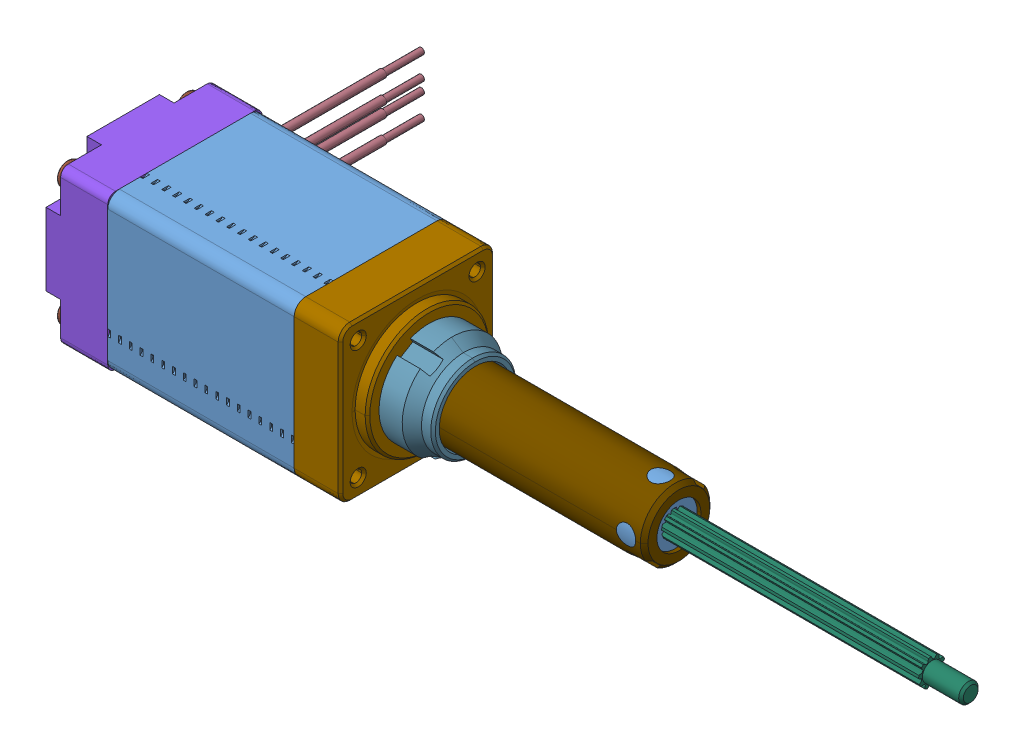
SolidWorks assembly 20NC38..31, configuration 默认. Lengths in mm.
Overall size (109.8 25.88 45.74).
31 component instances, 19 part files, 0 mates.
Components (placement in the parent):
- 20NC38..31.STEP-1: 20NC38..31.STEP [默认] at origin size (109.8 25.88 45.74)
  - 02-20-38.15________.STEP-1: 02-20-38.15________.STEP [默认] at origin size (39.65 25.88 45.74)
    - 02-20-38.STEP-1: 02-20-38.STEP [默认] at (20.075 0 0) x (0 0 1) z (-1 0 0) size (26.04 25.88 31.46)
      - 02-20-24.15_10-20-001-2.STEP-1: 02-20-24.15_10-20-001-2.STEP [默认] at origin size (20 20 24.15)
      - 13-20-8.5____.STEP-1: 13-20-8.5____.STEP [默认] at (0 0 16.075) x (0 1 0) z (0 0 -1) size (18.2 22.2 10.51)
      - 13-20-12.5______.STEP-1: 13-20-12.5______.STEP [默认] at (0 0 -14.575) x (0.707107 0.707107 0) z (0 0 1) size (18.3 18.3 15.8)
    - 03-20-008______38_______default.STEP-1: 03-20-008______38_______default.STEP [默认] at (3.8 0 0) x (1 0 0) z (0 0.78069 0.624918) size (32.3 16.26 16.27)
      - 06-20-008______38_________01-20-007-1.STEP-1: 06-20-008______38_________01-20-007-1.STEP [默认] at origin size (32.3 7 7)
      - 03-20-4.2-6YK_10-20-006-2.STEP-1: 03-20-4.2-6YK_10-20-006-2.STEP [默认] at (24.2 0 0) x (0 0.91534 0.402682) z (-1 0 0) size (12.06 12.08 4.2)
      - 10-20-001__________.STEP-1: 10-20-001__________.STEP [默认] at (16.9 0 0) x (0 0 1) z (-1 0 0) size (11.2 11.2 1.3)
      - 08-20-001______1_______07-20-001-1.STEP-1: 08-20-001______1_______07-20-001-1.STEP [默认] at (22.1 0 0) x (0 0 1) z (-1 0 0) size (11 11 1)
      - 08-20-001______1_______07-20-001-1.STEP-2: 08-20-001______1_______07-20-001-1.STEP [默认] at (11.4 0 0) x (0 0 1) z (-1 0 0) size (11 11 1)
      - 03-20-4.2-6YK_10-20-006-2.STEP-2: 03-20-4.2-6YK_10-20-006-2.STEP [默认] at (19 0 0) x (0 0.888249 0.459362) z (-1 0 0) size (12.06 12.08 4.2)
      - 03-20-4.2-6YK_10-20-006-2.STEP-3: 03-20-4.2-6YK_10-20-006-2.STEP [默认] at (13.5 0 0) x (0 0.91534 0.402682) z (-1 0 0) size (12.06 12.08 4.2)
      - 03-20-4.2-6YK_10-20-006-2.STEP-4: 03-20-4.2-6YK_10-20-006-2.STEP [默认] at (8.3 0 0) x (0 0.888249 0.459362) z (-1 0 0) size (12.06 12.08 4.2)
    - 01-20-003__20__________________.STEP-1: 01-20-003__20__________________.STEP [默认] at origin size (8.8 20 20)
    - 01-20-001__20__________________.STEP-1: 01-20-001__20__________________.STEP [默认] at (31.35 0 0) x (0 0 1) z (1 0 0) size (20 20 8.3)
    - 09-20-001____9X__5X4)_09-20-001.STEP-1: 09-20-001____9X__5X4)_09-20-001.STEP [默认] at (33.1 0 0) x (1 0 0) z (0 0.994502 0.104719) size (3 9 9)
    - 09-20-001____9X__5X4)_09-20-001.STEP-2: 09-20-001____9X__5X4)_09-20-001.STEP [默认] at (3.8 0 0) x (1 0 0) z (0 -0.49427 -0.869308) size (3 9 9)
    - 11-20-002__M2-37__20-42__.STEP-1: 11-20-002__M2-37__20-42__.STEP [默认] at (0.39 -7.7 7.7) x (0 0 -1) z (1 0 0) size (3 3 33)
    - 11-20-002__M2-37__20-42__.STEP-2: 11-20-002__M2-37__20-42__.STEP [默认] at (0.39 -7.7 -7.7) x (0 1 0) z (1 0 0) size (3 3 33)
    - 11-20-002__M2-37__20-42__.STEP-3: 11-20-002__M2-37__20-42__.STEP [默认] at (0.39 7.7 -7.7) x (0 0 1) z (1 0 0) size (3 3 33)
    - 11-20-002__M2-37__20-42__.STEP-4: 11-20-002__M2-37__20-42__.STEP [默认] at (0.39 7.7 7.7) x (0 -1 0) z (1 0 0) size (3 3 33)
    - 06-20-099__20___________20____________YK.STEP-1: 06-20-099__20___________20____________YK.STEP [默认] at (31.1 0 0) x (0 -0.624918 0.78069) z (-1 0 0) size (6.01 6.01 10)
    - 14-20-001__20-28____________________.STEP-1: 14-20-001__20-28____________________.STEP [默认] at (6.15 0 -8.6) x (0 -1 0) z (0 0 1) size (10.5 3.4 24.5)
  - 07-20-007__________________.STEP-1: 07-20-007__________________.STEP [默认] at (39.65 0 0) x (-1 0 0) z (0 -0.999857 -0.016895) size (6 12.92 13)
  - 07-20-013-2______________.STEP-1: 07-20-013-2______________.STEP [默认] at (68.4 0 0) x (0 -0.714016 0.700129) z (1 0 0) size (3.42 3.5 41.4)
  - 07-20-013-3______________.STEP-1: 07-20-013-3______________.STEP [默认] at (20.15 0 0) x (0 0.924225 0.381849) z (1 0 0) size (8 8 56.63)
  - 07-20-006__20______.STEP-1: 07-20-006__20______.STEP [默认] at (67.9 0 0) x (0 0.924225 0.381849) z (1 0 0) size (4.8 4.8 0.5)
  - 07-20-013-1__20_____________08-20-002-1.STEP-1: 07-20-013-1__20_____________08-20-002-1.STEP [默认] at (36.1 0 0) x (0 0.004204 -0.999991) z (1 0 0) size (9.01 9.01 35.91)
  - 07-20-002__20________________.STEP-1: 07-20-002__20________________.STEP [默认] at (69.65 0 0) x (0 0.004204 -0.999991) z (1 0 0) size (9.01 9.01 3.1)
